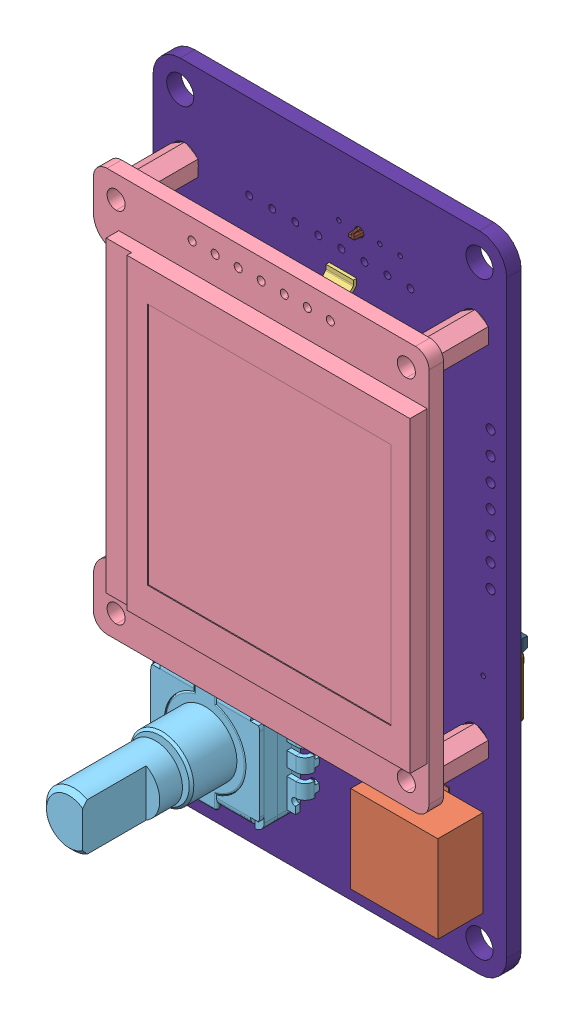
SolidWorks assembly AxxSolder, configuration Default. Lengths in mm.
Overall size (39 71 31.12).
38 component instances, 17 part files, 0 mates.
Components (placement in the parent):
- AxxSolder.step-1: AxxSolder.step [Default] at origin size (39 71 31.12)
  - 2N7002NXAKR.step-1: 2N7002NXAKR.step [Default] at (22.69 12.17 0.49) x (0 1 0) z (1 0 0) size (2.9 0.97 2.4)
    - COMPOUND.step-1: COMPOUND.step [Default] at origin size (2.9 0.97 2.4)
  - CMI-9653S-SMT-TR.step-1: CMI-9653S-SMT-TR.step [Default] at (31.75 11.25 1.65) x (0 -1 0) z (0 0 1) size (10.5 9.6 5.1)
    - COMPOUND-0.step-1: COMPOUND-0.step [Default] at origin size (10.5 9.6 5.1)
  - LD1117AS33TR.step-1: LD1117AS33TR.step [Default] at (21 56.25 1.65) x (0 1 0) z (0 0 1) size (7 6.5 1.9)
    - COMPOUND-1.step-1: COMPOUND-1.step [Default] at origin size (7 6.5 1.9)
  - 1_5inch-rgb-oled-module_asm-1110.step-1: 1_5inch-rgb-oled-module_asm-1110.step [Default] at (19.88 41.73 8.75) x (0 1 0) z (0 0 1) size (44.56 37.01 11.64)
    - COMPOUND-2.step-1: COMPOUND-2.step [Default] at origin size (44.56 37.01 11.64)
  - PEC11L-4xxxF-Sxxxx.step-1: PEC11L-4xxxF-Sxxxx.step [Default] at (10.3 11.5 5.65) x (0 1 0) z (0 0 1) size (12.82 15.5 22.5)
    - COMPOUND-3.step-1: COMPOUND-3.step [Default] at origin size (12.82 15.5 22.5)
  - TSR_2-2450.step-1: TSR_2-2450.step [Default] at (14.0177 56.84 -9.97) size (14 7.5 14.2)
    - SOLID.step-1: SOLID.step [Default] at origin size (14 7.5 14.2)
  - BAT54S,215.step-1: BAT54S,215.step [Default] at (18 46.68 1.15) x (0 1 0) z (-1 0 0) size (2.9 0.97 2.4)
    - COMPOUND-4.step-1: COMPOUND-4.step [Default] at origin size (2.9 0.97 2.4)
  - WSLP25122L500FEA.step-1: WSLP25122L500FEA.step [Default] at (14.5 34.75 -0.05) x (-1 0 0) z (0 0 -1) size (6.35 3.18 0.64)
    - COMPOUND-5.step-1: COMPOUND-5.step [Default] at origin size (6.35 3.18 0.64)
  - BAT54S,215.step-2: BAT54S,215.step [Default] at (31.475 29.68 1.15) x (0 1 0) z (-1 0 0) size (2.9 0.97 2.4)
    - COMPOUND-4.step-1: COMPOUND-4.step [Default] at origin size (2.9 0.97 2.4)
  - BAT54S,215.step-3: BAT54S,215.step [Default] at (18 49.93 1.15) x (0 1 0) z (-1 0 0) size (2.9 0.97 2.4)
    - COMPOUND-4.step-1: COMPOUND-4.step [Default] at origin size (2.9 0.97 2.4)
  - 3557-2.step-1: 3557-2.step [Default] at (31.21 36.51 6.27) x (-1 0 0) z (0 -1 0) size (19.82 10.17 6.74)
    - SHELL.step-1: SHELL.step [Default] at origin size (19.82 10.17 6.74)
  - TMP236AQDBZRQ1.step-1: TMP236AQDBZRQ1.step [Default] at (37.25 31.75 -0.05) x (0 -1 0) z (0 0 -1) size (2.54 2.92 1.01)
    - COMPOUND-6.step-1: COMPOUND-6.step [Default] at origin size (2.54 2.92 1.01)
  - testpin black 1mm.step-1: testpin black 1mm.step [Default] at (22.75 64.25 -0.05) x (-1 0 0) z (0 0 -1) size (2.37 2.55 7.69)
    - COMPOUND-7.step-1: COMPOUND-7.step [Default] at origin size (2.37 2.55 7.69)
  - PMEG6020ER,115.step-1: PMEG6020ER,115.step [Default] at (24.04 29.78 1.18) x (1 0 0) z (0 1 0) size (3.5 1.1 2)
    - COMPOUND-8.step-1: COMPOUND-8.step [Default] at origin size (3.5 1.1 2)
  - LTC4440AHMS8E-5#PBF.step-1: LTC4440AHMS8E-5#PBF.step [Default] at (23.25 34.5 -0.05) x (-1 0 0) z (0 0 -1) size (4.9 3 1.1)
    - COMPOUND-9.step-1: COMPOUND-9.step [Default] at origin size (4.9 3 1.1)
  - OPA2333AIDRBR.step-1: OPA2333AIDRBR.step [Default] at (17.6 43.2 -0.05) x (1 0 0) z (0 0 -1) size (3 3 0.78)
    - COMPOUND-10.step-1: COMPOUND-10.step [Default] at origin size (3 3 0.78)
  - BSC022N04LSATMA1.step-1: BSC022N04LSATMA1.step [Default] at (15.5 28.75 -0.05) x (1 0 0) z (0 0 -1) size (5.32 6.54 1.2)
    - COMPOUND-11.step-1: COMPOUND-11.step [Default] at origin size (5.32 6.54 1.2)
  - STM32G431KBT6.step-1: STM32G431KBT6.step [Default] at (28.5 48.25 -0.05) x (0 1 0) z (0 0 -1) size (9 9 1.6)
    - COMPOUND-12.step-1: COMPOUND-12.step [Default] at origin size (9 9 1.6)
  - AxxSolder PCB.step-1: AxxSolder PCB.step [Default] at origin size (39 71 1.6)
